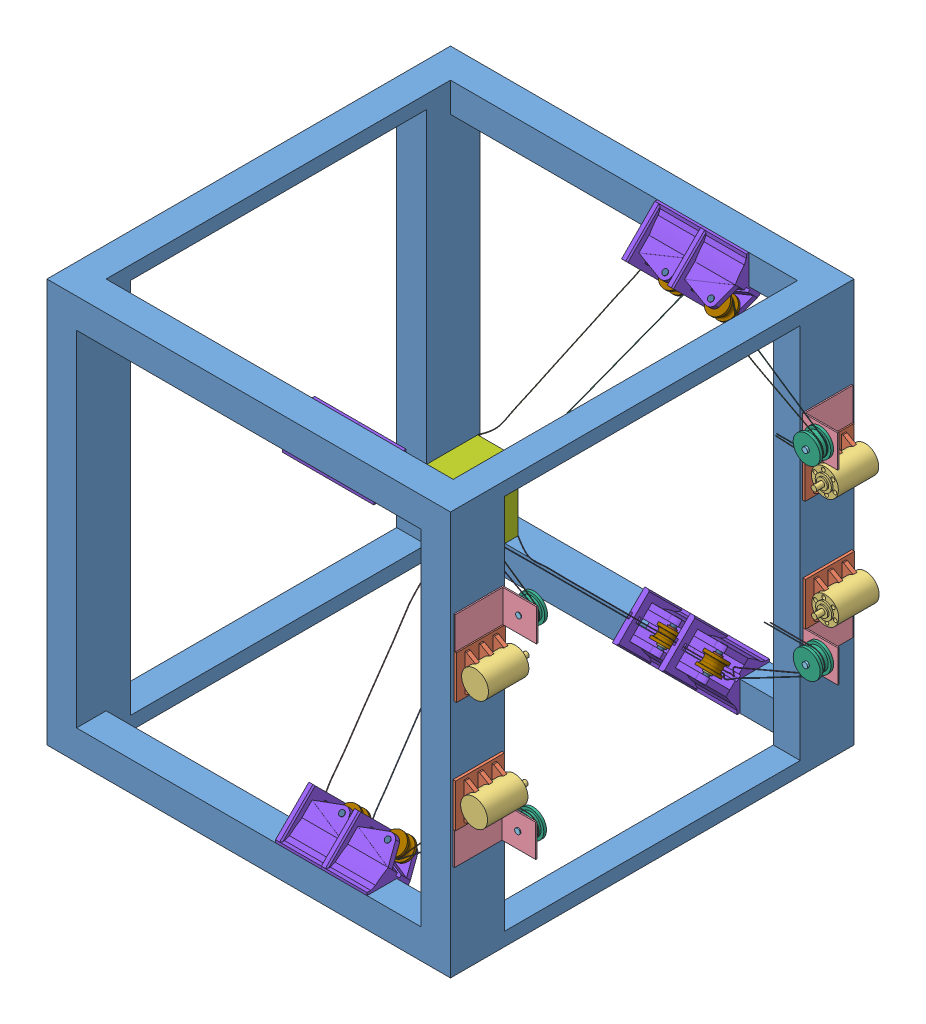
SolidWorks assembly 四自由度悬索机器人-粗装4, configuration 默认. Lengths in mm.
Overall size (1630.53 1500 1500).
86 component instances, 20 part files, 23 mates.
Components (placement in the parent):
- 框架-1: 框架 [默认] at (-869.4424 -713.1507 2250) size (1500 1500 1500)
- 驱动器-装配1-1: 驱动器-装配1 [默认] at (664.6049 -149.4407 667.2739) x (0 -1 0) z (0 0 1) size (280.09 130 239.56)
  - 驱动器--电机底座-1: 驱动器--电机底座 [默认] at (10.8985 -19.0474 121.978) size (160.09 50.28 181.98)
  - 驱动器-电机-1: 驱动器-电机 [默认] at (10.8985 30.9526 104.6663) x (0.931838 -0.362873 0) z (0 0 1) size (100 100 191)
  - 驱动器-滑轮组基座-1: 驱动器-滑轮组基座 [默认] at (90.9444 -34.0474 272.849) size (120 130 181.86)
  - 驱动器-定滑轮轴-1: 驱动器-定滑轮轴 [默认] at (150.9444 30.9526 265.5462) x (0.990128 -0.140168 0) z (0 0 1) size (20 20 65)
  - 驱动器-定滑轮-1: 驱动器-定滑轮 [默认] at (150.9167 30.9894 273.7821) x (0.990128 -0.140168 0) z (0 0 1) size (100 100 50)
- 驱动器-装配2-1: 驱动器-装配2 [默认] at (664.6049 262.8868 668.7376) x (0 -1 0) z (0 0 1) size (280.77 130.53 238.87)
  - 驱动器--电机底座-1: 驱动器--电机底座 [默认] at (10.8985 -19.0474 121.978) size (160.09 50.28 181.98)
  - 驱动器-电机-1: 驱动器-电机 [默认] at (10.8985 30.9526 104.6663) x (0.931838 -0.362873 0) z (0 0 1) size (100 100 191)
  - 驱动器-滑轮组基座-1: 驱动器-滑轮组基座 [默认] at (-189.8227 -33.5134 273.0905) size (120 130 181.86)
  - 驱动器-定滑轮轴-1: 驱动器-定滑轮轴 [默认] at (-129.7901 31.454 264.8545) size (20 20 65)
  - 驱动器-定滑轮-1: 驱动器-定滑轮 [默认] at (-129.8227 31.4866 273.0905) size (100 100 50)
- 驱动器-装配3-1: 驱动器-装配3 [默认] at (664.6049 -169.9542 2331.8379) x (0 1 0) z (0 0 -1) size (280.77 130.53 238.87)
  - 驱动器--电机底座-1: 驱动器--电机底座 [默认] at (10.8985 -19.0474 121.978) size (160.09 50.28 181.98)
  - 驱动器-电机-1: 驱动器-电机 [默认] at (10.8985 30.9526 104.6663) x (0.931838 -0.362873 0) z (0 0 1) size (100 100 191)
  - 驱动器-滑轮组基座-1: 驱动器-滑轮组基座 [默认] at (-189.8227 -33.5134 273.0905) size (120 130 181.86)
  - 驱动器-定滑轮轴-1: 驱动器-定滑轮轴 [默认] at (-129.7901 31.454 264.8545) size (20 20 65)
  - 驱动器-定滑轮-1: 驱动器-定滑轮 [默认] at (-129.8227 31.4866 273.0905) size (100 100 50)
- 驱动器-装配4-1: 驱动器-装配4 [默认] at (664.6049 241.4404 2328.4017) x (0 1 0) z (0 0 -1) size (280.09 130 239.56)
  - 驱动器--电机底座-1: 驱动器--电机底座 [默认] at (10.8985 -19.0474 121.978) size (160.09 50.28 181.98)
  - 驱动器-电机-1: 驱动器-电机 [默认] at (10.8985 30.9526 104.6663) x (0.931838 -0.362873 0) z (0 0 1) size (100 100 191)
  - 驱动器-滑轮组基座-1: 驱动器-滑轮组基座 [默认] at (90.9444 -34.0474 272.849) size (120 130 181.86)
  - 驱动器-定滑轮轴-1: 驱动器-定滑轮轴 [默认] at (150.9444 30.9526 265.5462) x (0.990128 -0.140168 0) z (0 0 1) size (20 20 65)
  - 驱动器-定滑轮-1: 驱动器-定滑轮 [默认] at (150.9167 30.9894 273.7821) x (0.990128 -0.140168 0) z (0 0 1) size (100 100 50)
- 执行器-1: 执行器 [默认] at (19.774 123.7995 1388.1997) x (0 -1 0) z (0 0 -1) size (250 150 200)
- 定滑轮组-装配1-2: 定滑轮组-装配1 [默认] at (151.3965 -782.1229 1166.7393) x (0 0 1) z (0 1 0) size (243.74 373.92 243.74)
  - 定滑轮-装配1-1: 定滑轮-装配1 [默认] at (-55.5304 53.8794 -79.4394) size (243.74 203.92 243.74)
    - 定滑轮-基座-1: 定滑轮-基座 [默认] at (-251.2089 -39.3736 258.4115) size (243.74 192.85 243.74)
    - 定滑轮-滚轮-1: 定滑轮-滚轮 [默认] at (-178.7162 65.1416 294.8732) x (0.51029 0.692249 0.51029) z (-0.707107 0 0.707107) size (80 80 50)
    - 定滑轮-轴-1: 定滑轮-轴 [默认] at (-153.8809 65.1416 270.0379) x (0.51029 0.692249 0.51029) z (-0.707107 0 0.707107) size (20 20 120)
    - 定滑轮-轴承1-1: 定滑轮-轴承1 [默认] at (-214.0716 65.1416 330.2286) x (0.51029 0.692249 0.51029) z (-0.707107 0 0.707107) size (30 30 5)
    - 定滑轮-轴承2-1: 定滑轮-轴承2 [默认] at (-175.1807 65.1416 291.3377) x (0.51029 0.692249 0.51029) z (-0.707107 0 0.707107) size (30 30 5)
  - 定滑轮-装配2-1: 定滑轮-装配2 [默认] at (-55.5304 -116.1206 -79.4394) size (243.74 203.92 243.74)
    - 定滑轮-基座-1: 定滑轮-基座 [默认] at (-251.2089 -39.3736 258.4115) size (243.74 192.85 243.74)
    - 定滑轮-滚轮-1: 定滑轮-滚轮 [默认] at (-178.7162 65.1416 294.8732) x (0.51029 0.692249 0.51029) z (-0.707107 0 0.707107) size (80 80 50)
    - 定滑轮-轴-1: 定滑轮-轴 [默认] at (-153.8809 65.1416 270.0379) x (0.51029 0.692249 0.51029) z (-0.707107 0 0.707107) size (20 20 120)
    - 定滑轮-轴承1-1: 定滑轮-轴承1 [默认] at (-214.0716 65.1416 330.2286) x (0.51029 0.692249 0.51029) z (-0.707107 0 0.707107) size (30 30 5)
    - 定滑轮-轴承2-1: 定滑轮-轴承2 [默认] at (-175.1807 65.1416 291.3377) x (0.51029 0.692249 0.51029) z (-0.707107 0 0.707107) size (30 30 5)
- 定滑轮组-装配2-1: 定滑轮组-装配2 [默认] at (155.9329 -296.4114 2318.9721) x (0 1 0) z (0 0 -1) size (243.74 373.92 243.74)
  - 定滑轮-装配1-1: 定滑轮-装配1 [默认] at (-55.5304 53.8794 -79.4394) size (243.74 203.92 243.74)
    - 定滑轮-基座-1: 定滑轮-基座 [默认] at (-251.2089 -39.3736 258.4115) size (243.74 192.85 243.74)
    - 定滑轮-滚轮-1: 定滑轮-滚轮 [默认] at (-178.7162 65.1416 294.8732) x (0.51029 0.692249 0.51029) z (-0.707107 0 0.707107) size (80 80 50)
    - 定滑轮-轴-1: 定滑轮-轴 [默认] at (-153.8809 65.1416 270.0379) x (0.51029 0.692249 0.51029) z (-0.707107 0 0.707107) size (20 20 120)
    - 定滑轮-轴承1-1: 定滑轮-轴承1 [默认] at (-214.0716 65.1416 330.2286) x (0.51029 0.692249 0.51029) z (-0.707107 0 0.707107) size (30 30 5)
    - 定滑轮-轴承2-1: 定滑轮-轴承2 [默认] at (-175.1807 65.1416 291.3377) x (0.51029 0.692249 0.51029) z (-0.707107 0 0.707107) size (30 30 5)
  - 定滑轮-装配2-1: 定滑轮-装配2 [默认] at (-55.5304 -116.1206 -79.4394) size (243.74 203.92 243.74)
    - 定滑轮-基座-1: 定滑轮-基座 [默认] at (-251.2089 -39.3736 258.4115) size (243.74 192.85 243.74)
    - 定滑轮-滚轮-1: 定滑轮-滚轮 [默认] at (-178.7162 65.1416 294.8732) x (0.51029 0.692249 0.51029) z (-0.707107 0 0.707107) size (80 80 50)
    - 定滑轮-轴-1: 定滑轮-轴 [默认] at (-153.8809 65.1416 270.0379) x (0.51029 0.692249 0.51029) z (-0.707107 0 0.707107) size (20 20 120)
    - 定滑轮-轴承1-1: 定滑轮-轴承1 [默认] at (-214.0716 65.1416 330.2286) x (0.51029 0.692249 0.51029) z (-0.707107 0 0.707107) size (30 30 5)
    - 定滑轮-轴承2-1: 定滑轮-轴承2 [默认] at (-175.1807 65.1416 291.3377) x (0.51029 0.692249 0.51029) z (-0.707107 0 0.707107) size (30 30 5)
- 定滑轮组-装配3-3: 定滑轮组-装配3 [默认] at (185.4984 370.1099 681.0279) x (0 -1 0) z (0 0 1) size (243.74 373.92 243.74)
  - 定滑轮-装配1-1: 定滑轮-装配1 [默认] at (-55.5304 53.8794 -79.4394) size (243.74 203.92 243.74)
    - 定滑轮-基座-1: 定滑轮-基座 [默认] at (-251.2089 -39.3736 258.4115) size (243.74 192.85 243.74)
    - 定滑轮-滚轮-1: 定滑轮-滚轮 [默认] at (-178.7162 65.1416 294.8732) x (0.51029 0.692249 0.51029) z (-0.707107 0 0.707107) size (80 80 50)
    - 定滑轮-轴-1: 定滑轮-轴 [默认] at (-153.8809 65.1416 270.0379) x (0.51029 0.692249 0.51029) z (-0.707107 0 0.707107) size (20 20 120)
    - 定滑轮-轴承1-1: 定滑轮-轴承1 [默认] at (-214.0716 65.1416 330.2286) x (0.51029 0.692249 0.51029) z (-0.707107 0 0.707107) size (30 30 5)
    - 定滑轮-轴承2-1: 定滑轮-轴承2 [默认] at (-175.1807 65.1416 291.3377) x (0.51029 0.692249 0.51029) z (-0.707107 0 0.707107) size (30 30 5)
  - 定滑轮-装配2-1: 定滑轮-装配2 [默认] at (-55.5304 -116.1206 -79.4394) size (243.74 203.92 243.74)
    - 定滑轮-基座-1: 定滑轮-基座 [默认] at (-251.2089 -39.3736 258.4115) size (243.74 192.85 243.74)
    - 定滑轮-滚轮-1: 定滑轮-滚轮 [默认] at (-178.7162 65.1416 294.8732) x (0.51029 0.692249 0.51029) z (-0.707107 0 0.707107) size (80 80 50)
    - 定滑轮-轴-1: 定滑轮-轴 [默认] at (-153.8809 65.1416 270.0379) x (0.51029 0.692249 0.51029) z (-0.707107 0 0.707107) size (20 20 120)
    - 定滑轮-轴承1-1: 定滑轮-轴承1 [默认] at (-214.0716 65.1416 330.2286) x (0.51029 0.692249 0.51029) z (-0.707107 0 0.707107) size (30 30 5)
    - 定滑轮-轴承2-1: 定滑轮-轴承2 [默认] at (-175.1807 65.1416 291.3377) x (0.51029 0.692249 0.51029) z (-0.707107 0 0.707107) size (30 30 5)
- 定滑轮组-装配4-2: 定滑轮组-装配4 [默认] at (180.9786 855.8214 1833.2607) x (0 0 -1) z (0 -1 0) size (243.74 373.92 243.74)
  - 定滑轮-装配1-1: 定滑轮-装配1 [默认] at (-55.5304 53.8794 -79.4394) size (243.74 203.92 243.74)
    - 定滑轮-基座-1: 定滑轮-基座 [默认] at (-251.2089 -39.3736 258.4115) size (243.74 192.85 243.74)
    - 定滑轮-滚轮-1: 定滑轮-滚轮 [默认] at (-178.7162 65.1416 294.8732) x (0.51029 0.692249 0.51029) z (-0.707107 0 0.707107) size (80 80 50)
    - 定滑轮-轴-1: 定滑轮-轴 [默认] at (-153.8809 65.1416 270.0379) x (0.51029 0.692249 0.51029) z (-0.707107 0 0.707107) size (20 20 120)
    - 定滑轮-轴承1-1: 定滑轮-轴承1 [默认] at (-214.0716 65.1416 330.2286) x (0.51029 0.692249 0.51029) z (-0.707107 0 0.707107) size (30 30 5)
    - 定滑轮-轴承2-1: 定滑轮-轴承2 [默认] at (-175.1807 65.1416 291.3377) x (0.51029 0.692249 0.51029) z (-0.707107 0 0.707107) size (30 30 5)
  - 定滑轮-装配2-1: 定滑轮-装配2 [默认] at (-55.5304 -116.1206 -79.4394) size (243.74 203.92 243.74)
    - 定滑轮-基座-1: 定滑轮-基座 [默认] at (-251.2089 -39.3736 258.4115) size (243.74 192.85 243.74)
    - 定滑轮-滚轮-1: 定滑轮-滚轮 [默认] at (-178.7162 65.1416 294.8732) x (0.51029 0.692249 0.51029) z (-0.707107 0 0.707107) size (80 80 50)
    - 定滑轮-轴-1: 定滑轮-轴 [默认] at (-153.8809 65.1416 270.0379) x (0.51029 0.692249 0.51029) z (-0.707107 0 0.707107) size (20 20 120)
    - 定滑轮-轴承1-1: 定滑轮-轴承1 [默认] at (-214.0716 65.1416 330.2286) x (0.51029 0.692249 0.51029) z (-0.707107 0 0.707107) size (30 30 5)
    - 定滑轮-轴承2-1: 定滑轮-轴承2 [默认] at (-175.1807 65.1416 291.3377) x (0.51029 0.692249 0.51029) z (-0.707107 0 0.707107) size (30 30 5)
- 绳1-1: 绳1 [默认] at origin size (718.73 546.46 497)
- 绳2-1: 绳2 [默认] at origin size (868.75 552.4 523.29)
- 绳3-1: 绳3 [默认] at origin size (723.76 427.02 492.19)
- 绳4-1: 绳4 [默认] at origin size (871.45 439.72 502.99)
- 绳5-1: 绳5 [默认] at origin size (743.88 445.89 515.69)
- 绳6-1: 绳6 [默认] at origin size (893.72 467.35 516.45)
- 绳7-1: 绳7 [默认] at origin size (721.1 554.76 527.15)
- 绳8-1: 绳8 [默认] at origin size (871.07 547.31 524.26)
Mates (geometry in assembly coordinates):
- 平行35: parallel: plane of assembly; plane of assembly; plane of 框架-1 through (520.5576 676.8493 2250) normal (-1 0 0); plane of 执行器-1 through (19.774 123.7995 1388.1997) normal (1 0 0)
- 平行36: parallel: plane of assembly; plane of assembly; plane of 框架-1 through (520.5576 676.8493 2250) normal (0 -1 0); plane of 执行器-1 through (-130.226 223.7995 1588.1997) normal (0 1 0)
- 平行37: parallel: plane of assembly; plane of assembly; plane of 框架-1 through (530.5576 786.8493 2140) normal (0 0 -1); plane of 执行器-1 through (-130.226 223.7995 1588.1997) normal (0 0 1)
- 平行38: parallel: plane of assembly; plane of assembly; plane of 框架-1 through (520.5576 676.8493 2250) normal (-1 0 0); plane of 定滑轮组-装配1-2/定滑轮-装配1-1/定滑轮-基座-1 through (315.9023 -603.1507 860) normal (1 0 0)
- 重合43: coincident: plane of assembly; plane of assembly; plane of 框架-1 through (530.5576 786.8493 860) normal (0 0 1); plane of 定滑轮组-装配1-2/定滑轮-装配1-1/定滑轮-基座-1 through (315.9023 -603.1507 860) normal (0 0 -1)
- 重合44: coincident: plane of assembly; plane of assembly; plane of 框架-1 through (520.5576 -603.1507 2250) normal (0 1 0); plane of 定滑轮组-装配1-2/定滑轮-装配1-1/定滑轮-基座-1 through (315.9023 -603.1507 750) normal (0 -1 0)
- 平行39: parallel: plane of 框架-1 through (520.5576 676.8493 2250) normal (-1 0 0); plane of 定滑轮组-装配2-1/定滑轮-装配1-1/定滑轮-基座-1 through (320.4388 -603.1507 2140) normal (1 0 0)
- 重合47: coincident: plane of 框架-1 through (520.5576 -603.1507 2250) normal (0 1 0); plane of 定滑轮组-装配2-1/定滑轮-装配1-1/定滑轮-基座-1 through (320.4388 -603.1507 2140) normal (0 -1 0)
- 重合48: coincident: plane of 框架-1 through (530.5576 786.8493 2140) normal (0 0 -1); plane of 定滑轮组-装配2-1/定滑轮-装配1-1/定滑轮-基座-1 through (320.4388 -713.1507 2140) normal (0 0 1)
- 平行41: parallel: plane of 框架-1 through (530.5576 786.8493 2140) normal (-1 0 0); plane of 定滑轮组-装配3-3/定滑轮-装配1-1/定滑轮-基座-1 through (350.0042 676.8493 860) normal (1 0 0)
- 重合52: coincident: plane of 框架-1 through (520.5576 676.8493 2250) normal (0 -1 0); plane of 定滑轮组-装配3-3/定滑轮-装配1-1/定滑轮-基座-1 through (350.0042 676.8493 860) normal (0 1 0)
- 重合53: coincident: plane of 框架-1 through (530.5576 786.8493 860) normal (0 0 1); plane of 定滑轮组-装配3-3/定滑轮-装配1-1/定滑轮-基座-1 through (350.0042 786.8493 860) normal (0 0 -1)
- 平行42: parallel: plane of 框架-1 through (520.5576 676.8493 2250) normal (-1 0 0); plane of 定滑轮组-装配4-2/定滑轮-装配1-1/定滑轮-基座-1 through (345.4844 676.8493 2140) normal (1 0 0)
- 重合55: coincident: plane of 框架-1 through (520.5576 676.8493 2250) normal (0 -1 0); plane of 定滑轮组-装配4-2/定滑轮-装配1-1/定滑轮-基座-1 through (345.4844 676.8493 2250) normal (0 1 0)
- 重合57: coincident: plane of 框架-1 through (530.5576 786.8493 2140) normal (0 0 -1); plane of 定滑轮组-装配4-2/定滑轮-装配1-1/定滑轮-基座-1 through (345.4844 676.8493 2140) normal (0 0 1)
- 重合62: coincident: plane of assembly; plane of assembly; plane of 框架-1 through (630.5576 786.8493 2250) normal (1 0 0); plane of 驱动器-装配1-1/驱动器--电机底座-1 through (630.5576 -160.3393 789.2519) normal (-1 0 0)
- 平行43: parallel: line of assembly; line of assembly; line of 框架-1 through (630.5576 786.8493 750) axis (0 -1 0); line of 驱动器-装配1-1/驱动器--电机底座-1 through (630.5576 -240.3851 758.2629) axis (0 1 0)
- 重合65: coincident: plane of 框架-1 through (630.5576 786.8493 2250) normal (1 0 0); plane of 驱动器-装配2-1/驱动器--电机底座-1 through (630.5576 251.9882 790.7156) normal (-1 0 0)
- 平行44: parallel: line of 框架-1 through (630.5576 786.8493 750) axis (0 -1 0); line of 驱动器-装配2-1/驱动器--电机底座-1 through (630.5576 171.9424 759.7266) axis (0 1 0)
- 重合68: coincident: plane of 框架-1 through (630.5576 786.8493 2250) normal (1 0 0); plane of 驱动器-装配3-1/驱动器--电机底座-1 through (630.5576 -159.0557 2209.8599) normal (-1 0 0)
- 平行45: parallel: line of 框架-1 through (630.5576 786.8493 2250) axis (0 -1 0); line of 驱动器-装配3-1/驱动器--电机底座-1 through (630.5576 -79.0098 2240.8489) axis (0 -1 0)
- 重合71: coincident: plane of assembly; plane of assembly; plane of 框架-1 through (630.5576 786.8493 2250) normal (1 0 0); plane of 驱动器-装配4-1/驱动器-滑轮组基座-1 through (630.5576 452.3848 2055.5527) normal (-1 0 0)
- 平行46: parallel: line of assembly; line of assembly; line of 框架-1 through (630.5576 786.8493 2250) axis (0 -1 0); line of 驱动器-装配4-1/驱动器-滑轮组基座-1 through (630.5576 452.3848 2237.4127) axis (0 -1 0)
